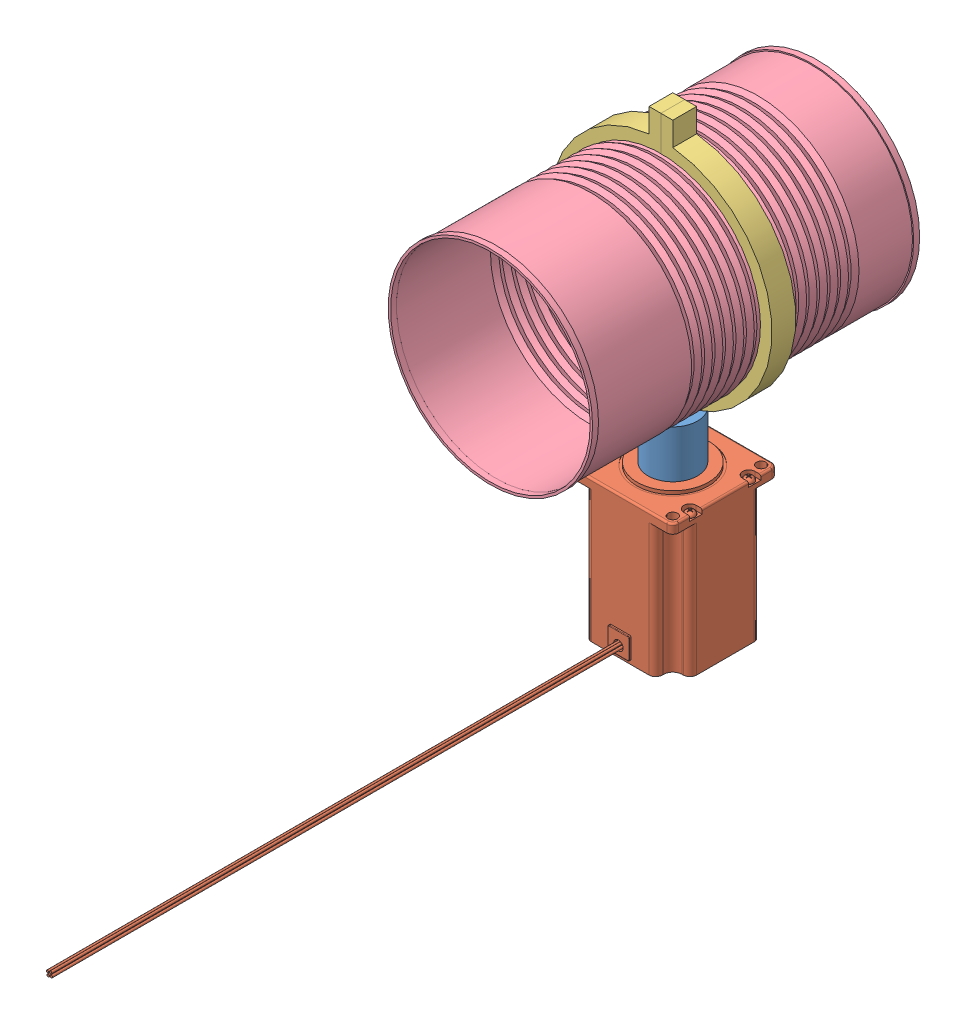
SolidWorks assembly Rotating Cantenna, configuration Default. Lengths in mm.
Overall size (118.68 257.2 410.06).
5 component instances, 4 part files, 9 mates.
Components (placement in the parent):
- Mast to Shaft Adapter-1: Mast to Shaft Adapter [Default] at (-227.2544 6.6981 -48.5008) size (26.42 25.4 26.42)
- 5718L-XXD_Standard-1: 5718L-XXD_Standard [Default] at (-227.2544 -5.7987 -48.5008) x (1 0 0) z (0 1 0) size (56.06 360.86 112.03)
- Cantenna_Clamp-1: Cantenna_Clamp [Default] at (-227.2544 99.2267 -54.8508) x (1 0 0) z (0 -1 0) size (59.34 12.7 143.4)
- Cantenna_Clamp-2: Cantenna_Clamp [Default] at (-227.2544 99.2267 -42.1508) x (-1 0 0) z (0 -1 0) size (59.34 12.7 143.4)
- Cantenna Frame-1: Cantenna Frame [Default] at (-227.2544 99.2267 -121.9214) x (1 0 0) z (0 -1 0) size (109.18 174.62 109.18)
Mates (geometry in assembly coordinates):
- Concentric7: concentric anti-aligned: cylinder of Mast to Shaft Adapter-1 through (-227.2544 32.0981 -48.5008) axis (0 -1 0) radius 3.175; cylinder of 5718L-XXD_Standard-1 through (-227.2544 4.1583 -48.5008) axis (0 1 0) radius 3.175
- Coincident9: coincident anti-aligned: plane of Mast to Shaft Adapter-1 through (-227.2544 6.6981 -48.5008) normal (0 -1 0); plane of 5718L-XXD_Standard-1 through (-227.2544 6.6981 -48.5008) normal (0 1 0)
- Coincident10: coincident anti-aligned: plane of Mast to Shaft Adapter-1 through (-227.2544 27.5261 -48.5008) normal (0 1 0); plane of Cantenna_Clamp-1 through (-227.2544 27.5261 -42.1508) normal (0 -1 0)
- Coincident11: coincident anti-aligned: plane of Mast to Shaft Adapter-1 through (-220.9044 27.5261 -42.1508) normal (-1 0 0); plane of Cantenna_Clamp-1 through (-220.9044 27.5261 -42.1508) normal (1 0 0)
- Coincident12: coincident anti-aligned: plane of Mast to Shaft Adapter-1 through (-233.6044 27.5261 -54.8508) normal (0 0 1); plane of Cantenna_Clamp-1 through (-227.2544 99.2267 -54.8508) normal (0 0 -1)
- Coincident15: coincident anti-aligned: plane of Mast to Shaft Adapter-1 through (-227.2544 27.5261 -48.5008) normal (0 1 0); plane of Cantenna_Clamp-2 through (-227.2544 27.5261 -54.8508) normal (0 -1 0)
- Coincident16: coincident anti-aligned: plane of Mast to Shaft Adapter-1 through (-233.6044 27.5261 -42.1508) normal (1 0 0); plane of Cantenna_Clamp-2 through (-233.6044 27.5261 -54.8508) normal (-1 0 0)
- Coincident17: coincident anti-aligned: plane of Mast to Shaft Adapter-1 through (-233.6044 27.5261 -54.8508) normal (0 0 1); plane of Cantenna_Clamp-2 through (-227.2544 99.2267 -54.8508) normal (0 0 -1)
- Concentric12: concentric aligned: cylinder of Cantenna_Clamp-1 through (-227.2544 99.2267 -42.1508) axis (0 0 -1) radius 52.9913; cylinder of Cantenna Frame-1 through (-227.2544 99.2267 -1121.9214) axis (0 0 -1) radius 53.9425
